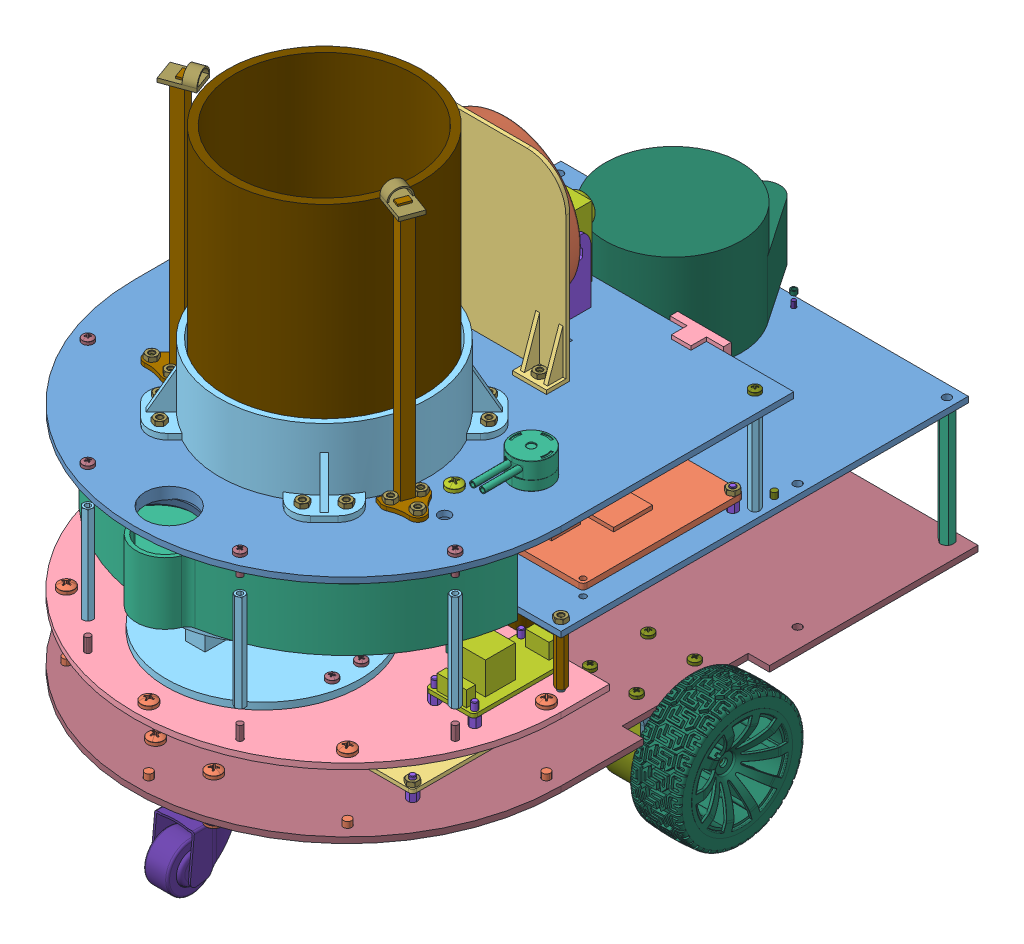
SolidWorks assembly 总装配, configuration 默认. Lengths in mm.
Overall size (259.72 318.06 332.82).
184 component instances, 44 part files, 87 mates.
Components (placement in the parent):
- 中层结构装配-1: 中层结构装配 [默认] at (0 31.5 0) size (220 94.26 332.82)
  - 支撑件_上部-1: 支撑件_上部 [默认] at (0 31 0) size (210 3 210)
  - stm32开发板51_2×82_8-1: stm32开发板51_2×82_8 [默认] at (72.18 39 -65) size (51.24 5 82.8)
  - 6490开发板100×130×39.25-1: 6490开发板100×130×39.25 [默认] at (-40 39 -65) x (0 0 -1) z (1 0 0) size (107 40.25 130)
  - 支撑件_最底部-2: 支撑件_最底部 [默认] at origin size (220 3 135)
  - 压力传感器100-1: 压力传感器100 [默认] at (0 6 43.5) x (0 0 -1) z (1 0 0) size (100 38.5 100)
  - 蓄水容器-1: 蓄水容器 [默认] at (0 44.5 60) size (194.98 32 99)
  - 继电器50x25x18.5-1: 继电器50x25x18.5 [默认] at (83.25 8 5.75) x (0 0 1) z (-1 0 0) size (50 18.5 25)
  - 单通六角螺柱M3-L5]-1: 单通六角螺柱M3-L5] [默认] at (-100 45 -110) x (0 -1 0) z (0 0 1) size (11 5.32 5.32)
  - 单通六角螺柱M3-L5]-2: 单通六角螺柱M3-L5] [默认] at (-100 45 -20) x (0 -1 0) z (0.188455 0 0.982082) size (11 5.32 5.32)
  - 单通六角螺柱M3-L5]-3: 单通六角螺柱M3-L5] [默认] at (20 45 -110) x (0 -1 0) z (0.395734 0 0.918365) size (11 5.32 5.32)
  - 单通六角螺柱M3-L5]-4: 单通六角螺柱M3-L5] [默认] at (20 45 -20) x (0 -1 0) z (0.6 0 0.8) size (11 5.32 5.32)
  - 双通六角螺柱M3-L25]-1: 双通六角螺柱M3-L25] [默认] at (-100 17 -10) x (0 1 0) z (-0.516013 0 0.856581) size (25.01 5.44 5.43)
  - 双通六角螺柱M3-L25]-2: 双通六角螺柱M3-L25] [默认] at (100 17 -10) x (0 1 0) z (-0.345341 0 0.938477) size (25.01 5.44 5.43)
  - 双通六角螺柱M3-L25]-4: 双通六角螺柱M3-L25] [默认] at (0 17 -10) x (0 1 0) z (-0.345341 0 0.938477) size (25.01 5.44 5.43)
  - 蓄水容器盖子-1: 蓄水容器盖子 [默认] at (0 77.4896 10) x (1 0 0) z (0 0 -1) size (194.98 5 80)
  - GB╱T 818-2016[十字槽盘头螺钉M3×4]-1: GB╱T 818-2016[十字槽盘头螺钉M3×4] [默认] at (-100 28.6 -110) x (0 1 0) z (0 0 1) size (6.35 5.6 5.6)
  - 六角螺母 SLMNA[SLMNA-M3]-1: 六角螺母 SLMNA[SLMNA-M3] [默认] at (-100 42 -110) x (1 0 0) z (0 1 0) size (5.5 6.35 2.41)
  - GB╱T 818-2016[十字槽盘头螺钉M3×4]-2: GB╱T 818-2016[十字槽盘头螺钉M3×4] [默认] at (-100 28.6 -20) x (0 1 0) z (0.188455 0 0.982082) size (6.35 5.6 5.6)
  - 六角螺母 SLMNA[SLMNA-M3]-2: 六角螺母 SLMNA[SLMNA-M3] [默认] at (-100 42 -20) x (0.982082 0 -0.188455) z (0 1 0) size (5.5 6.35 2.41)
  - GB╱T 818-2016[十字槽盘头螺钉M3×4]-4: GB╱T 818-2016[十字槽盘头螺钉M3×4] [默认] at (20 28.6 -110) x (0 1 0) z (0.395734 0 0.918365) size (6.35 5.6 5.6)
  - 六角螺母 SLMNA[SLMNA-M3]-4: 六角螺母 SLMNA[SLMNA-M3] [默认] at (20 42 -110) x (0.918365 0 -0.395734) z (0 1 0) size (5.5 6.35 2.41)
  - GB╱T 818-2016[十字槽盘头螺钉M3×4]-6: GB╱T 818-2016[十字槽盘头螺钉M3×4] [默认] at (20 28.6 -20) x (0 1 0) z (0.6 0 0.8) size (6.35 5.6 5.6)
  - 六角螺母 SLMNA[SLMNA-M3]-6: 六角螺母 SLMNA[SLMNA-M3] [默认] at (20 42 -20) x (0.8 0 -0.6) z (0 1 0) size (5.5 6.35 2.41)
  - GB╱T 818-2016[十字槽盘头螺钉M3×10]-1: GB╱T 818-2016[十字槽盘头螺钉M3×10] [默认] at (43 11.9 36) x (0 -1 0) z (-0.546944 0 0.837169) size (12.35 5.6 5.6)
  - GB╱T 818-2016[十字槽盘头螺钉M3×10]-2: GB╱T 818-2016[十字槽盘头螺钉M3×10] [默认] at (43 11.9 51) x (0 -1 0) z (-0.379375 0 0.925243) size (12.35 5.6 5.6)
  - GB╱T 818-2016[十字槽盘头螺钉M3×8]-2: GB╱T 818-2016[十字槽盘头螺钉M3×8] [默认] at (100 -2.4 -10) x (0 1 0) z (0.546944 0 -0.837169) size (10.35 5.6 5.6)
  - 六角螺母 SLMNA[SLMNA-M3]-9: 六角螺母 SLMNA[SLMNA-M3] [默认] at (100 34 -10) x (1 0 0) z (0 1 0) size (5.5 6.35 2.41)
  - 六角螺母 SLMNA[SLMNA-M3]-10: 六角螺母 SLMNA[SLMNA-M3] [默认] at (0 34 -10) x (0.982082 0 -0.188455) z (0 1 0) size (5.5 6.35 2.41)
  - GB╱T 818-2016[十字槽盘头螺钉M3×8]-3: GB╱T 818-2016[十字槽盘头螺钉M3×8] [默认] at (0 -2.4 -10) x (0 1 0) z (0.379375 0 -0.925243) size (10.35 5.6 5.6)
  - 六角螺母 SLMNA[SLMNA-M3]-14: 六角螺母 SLMNA[SLMNA-M3] [默认] at (-100 34 -10) x (0.92897 0 -0.370156) z (0 1 0) size (5.5 6.35 2.41)
  - GB╱T 818-2016[十字槽盘头螺钉M3×8]-6: GB╱T 818-2016[十字槽盘头螺钉M3×8] [默认] at (-100 -2.4 -10) x (0 1 0) z (0.198211 0 -0.980159) size (10.35 5.6 5.6)
  - 单通六角螺柱M3-L5]-5: 单通六角螺柱M3-L5] [默认] at (93.5 14 28) x (0 -1 0) z (-0.997819 0 -0.066013) size (11 5.32 5.32)
  - 单通六角螺柱M3-L5]-6: 单通六角螺柱M3-L5] [默认] at (73 14 28) x (0 -1 0) z (-0.99238 0 0.123213) size (11 5.32 5.32)
  - 单通六角螺柱M3-L5]-7: 单通六角螺柱M3-L5] [默认] at (93.5 14 -16.5) x (0 -1 0) z (-0.942486 0 0.334247) size (11 5.32 5.32)
  - 单通六角螺柱M3-L5]-8: 单通六角螺柱M3-L5] [默认] at (73 14 -16.5) x (0 -1 0) z (-0.837863 0 0.545881) size (11 5.32 5.32)
  - 雷达-2: 雷达 [默认] at (0 36.9114 -167.8168) x (0 0 -1) z (1 0 0) size (90 52 70)
  - 单通六角螺柱M3-L5]-10: 单通六角螺柱M3-L5] [默认] at (95 45 -103.6) x (0 -1 0) z (-0.546944 0 0.837169) size (11 5.32 5.32)
  - 六角螺母 SLMNA[SLMNA-M3]-15: 六角螺母 SLMNA[SLMNA-M3] [默认] at (95 44.4 -103.6) x (1 0 0) z (0 -1 0) size (5.5 6.35 2.41)
  - GB╱T 818-2016[十字槽盘头螺钉M3×6]-1: GB╱T 818-2016[十字槽盘头螺钉M3×6] [默认] at (95 28.6 -103.6) x (0 1 0) z (0 0 1) size (8.35 5.6 5.6)
  - GB╱T 818-2016[十字槽盘头螺钉M2×6]-1: GB╱T 818-2016[十字槽盘头螺钉M2×6] [默认] at (20 29.4 -210) x (0 1 0) z (-0.975796 0 -0.218684) size (7.56 4 4)
- 上层支撑结构-1: 上层支撑结构 [默认] at (0 116.5 0) size (220 164.3 234)
  - 花盆100×100×130-1: 花盆100×100×130 [默认] at (0 1 12) size (100 130 100)
  - 支撑件_最顶部-1: 支撑件_最顶部 [默认] x (-1 0 0) z (0 0 1) size (220 6 230)
  - 一体化麦-1: 一体化麦 [默认] at (0 49.5771 -67) x (1 0 0) z (0 1 0) size (88 15 88)
  - 上层竖直安装版-1: 上层竖直安装版 [默认] at (0 48.5 -67) size (95 95 12)
  - 0.96寸led大概-1: 0.96寸led大概 [默认] at (60 -10.65 -120) x (-1 0 0) z (0 0 -1) size (27.6 27.3 12)
  - 0.96寸led大概-3: 0.96寸led大概 [默认] at (-60 -10.65 -120) x (-1 0 0) z (0 0 -1) size (27.6 27.3 12)
  - 花盆支撑-1: 花盆支撑 [默认] at (-36.7696 1 48.7696) x (0.707107 0 -0.707107) z (0.707107 0 0.707107) size (134 35 134)
  - 蠕动泵-1: 蠕动泵 [默认] at (20.9584 -7.5 -18.6981) x (0 0 1) z (0 1 0) size (38.31 20 40.3)
  - 相机-1: 相机 [默认] at (0 28.3524 -102.4535) x (-1 0 0) z (0 0 -1) size (36 36 25.5)
  - 相机支架-1: 相机支架 [默认] at (0 1 -100) size (40.08 35.04 25)
  - 花盆引导架-1: 花盆引导架 [默认] at (62 1 30) x (0.939693 0 0.34202) z (-0.34202 0 0.939693) size (18.5 133 20.12)
  - 花盆引导架-2: 花盆引导架 [默认] at (-62 1 30) x (-0.939693 0 0.34202) z (-0.34202 0 -0.939693) size (18.5 133 20.12)
  - GB╱T 818-2016[十字槽盘头螺钉M3×6]-1: GB╱T 818-2016[十字槽盘头螺钉M3×6] [默认] at (68.5778 -4.4 32.3941) x (0 1 0) z (0 0 1) size (8.35 5.6 5.6)
  - GB╱T 818-2016[十字槽盘头螺钉M3×6]-2: GB╱T 818-2016[十字槽盘头螺钉M3×6] [默认] at (56.6377 -4.4 34.4995) x (0 1 0) z (0.188455 0 0.982082) size (8.35 5.6 5.6)
  - GB╱T 818-2016[十字槽盘头螺钉M3×6]-5: GB╱T 818-2016[十字槽盘头螺钉M3×6] [默认] at (60.7845 -4.4 23.1063) x (0 1 0) z (0.370156 0 0.92897) size (8.35 5.6 5.6)
  - GB╱T 818-2016[十字槽盘头螺钉M3×6]-7: GB╱T 818-2016[十字槽盘头螺钉M3×6] [默认] at (-56.6377 -4.4 34.4995) x (0 1 0) z (0.561714 0 0.827332) size (8.35 5.6 5.6)
  - GB╱T 818-2016[十字槽盘头螺钉M3×6]-10: GB╱T 818-2016[十字槽盘头螺钉M3×6] [默认] at (-68.5778 -4.4 32.3941) x (0 1 0) z (0.707564 0 0.70665) size (8.35 5.6 5.6)
  - GB╱T 818-2016[十字槽盘头螺钉M3×6]-12: GB╱T 818-2016[十字槽盘头螺钉M3×6] [默认] at (-60.7845 -4.4 23.1063) x (0 1 0) z (0.843262 0 0.537503) size (8.35 5.6 5.6)
  - GB╱T 818-2016[十字槽盘头螺钉M3×6]-14: GB╱T 818-2016[十字槽盘头螺钉M3×6] [默认] at (-36.7696 -4.4 60.0833) x (0 1 0) z (0.94577 0 0.324837) size (8.35 5.6 5.6)
  - GB╱T 818-2016[十字槽盘头螺钉M3×6]-16: GB╱T 818-2016[十字槽盘头螺钉M3×6] [默认] at (-48.0833 -4.4 48.7696) x (0 1 0) z (0.995978 0 0.089595) size (8.35 5.6 5.6)
  - GB╱T 818-2016[十字槽盘头螺钉M3×6]-18: GB╱T 818-2016[十字槽盘头螺钉M3×6] [默认] at (-48.0833 -4.4 -24.7696) x (0 1 0) z (0.990656 0 -0.136386) size (8.35 5.6 5.6)
  - GB╱T 818-2016[十字槽盘头螺钉M3×6]-20: GB╱T 818-2016[十字槽盘头螺钉M3×6] [默认] at (-36.7696 -4.4 -36.0833) x (0 1 0) z (0.100159 0 0.994971) size (8.35 5.6 5.6)
  - GB╱T 818-2016[十字槽盘头螺钉M3×6]-23: GB╱T 818-2016[十字槽盘头螺钉M3×6] [默认] at (36.7696 -4.4 -36.0833) x (0 1 0) z (0.888841 0 -0.458216) size (8.35 5.6 5.6)
  - GB╱T 818-2016[十字槽盘头螺钉M3×6]-25: GB╱T 818-2016[十字槽盘头螺钉M3×6] [默认] at (48.0833 -4.4 -24.7696) x (0 1 0) z (0.844013 0 -0.536322) size (8.35 5.6 5.6)
  - GB╱T 818-2016[十字槽盘头螺钉M3×6]-27: GB╱T 818-2016[十字槽盘头螺钉M3×6] [默认] at (36.7696 -4.4 60.0833) x (0 1 0) z (0.827332 0 -0.561714) size (8.35 5.6 5.6)
  - GB╱T 818-2016[十字槽盘头螺钉M3×6]-29: GB╱T 818-2016[十字槽盘头螺钉M3×6] [默认] at (48.0833 -4.4 48.7696) x (0 1 0) z (0.844013 0 -0.536322) size (8.35 5.6 5.6)
  - 六角螺母 SLMNA[SLMNA-M3]-1: 六角螺母 SLMNA[SLMNA-M3] [默认] at (-48.0833 6.4 48.7696) x (1 0 0) z (0 -1 0) size (5.5 6.35 2.41)
  - 六角螺母 SLMNA[SLMNA-M3]-2: 六角螺母 SLMNA[SLMNA-M3] [默认] at (-36.7696 6.4 60.0833) x (0.982082 0 -0.188455) z (0 -1 0) size (5.5 6.35 2.41)
  - 六角螺母 SLMNA[SLMNA-M3]-4: 六角螺母 SLMNA[SLMNA-M3] [默认] at (-68.5778 5.4 32.3941) x (0.918365 0 -0.395734) z (0 -1 0) size (5.5 6.35 2.41)
  - 六角螺母 SLMNA[SLMNA-M3]-6: 六角螺母 SLMNA[SLMNA-M3] [默认] at (-60.7845 5.4 23.1063) x (0.8 0 -0.6) z (0 -1 0) size (5.5 6.35 2.41)
  - 六角螺母 SLMNA[SLMNA-M3]-8: 六角螺母 SLMNA[SLMNA-M3] [默认] at (-56.6377 5.4 34.4995) x (0.63358 0 -0.773678) z (0 -1 0) size (5.5 6.35 2.41)
  - 六角螺母 SLMNA[SLMNA-M3]-10: 六角螺母 SLMNA[SLMNA-M3] [默认] at (56.6377 5.4 34.4995) x (0.443629 0 -0.896211) z (0 -1 0) size (5.5 6.35 2.41)
  - 六角螺母 SLMNA[SLMNA-M3]-12: 六角螺母 SLMNA[SLMNA-M3] [默认] at (68.5778 5.4 32.3941) x (0.263225 0 -0.964735) z (0 -1 0) size (5.5 6.35 2.41)
  - 六角螺母 SLMNA[SLMNA-M3]-14: 六角螺母 SLMNA[SLMNA-M3] [默认] at (60.7845 5.4 23.1063) x (0.120178 0 -0.992752) z (0 -1 0) size (5.5 6.35 2.41)
  - 六角螺母 SLMNA[SLMNA-M3]-16: 六角螺母 SLMNA[SLMNA-M3] [默认] at (48.0833 6.4 48.7696) x (0.030377 0 -0.999538) z (0 -1 0) size (5.5 6.35 2.41)
  - 六角螺母 SLMNA[SLMNA-M3]-18: 六角螺母 SLMNA[SLMNA-M3] [默认] at (36.7696 6.4 60.0833) x (0 0 -1) z (0 -1 0) size (5.5 6.35 2.41)
  - 六角螺母 SLMNA[SLMNA-M3]-20: 六角螺母 SLMNA[SLMNA-M3] [默认] at (48.0833 6.4 -24.7696) x (0.030377 0 -0.999538) z (0 -1 0) size (5.5 6.35 2.41)
  - 六角螺母 SLMNA[SLMNA-M3]-22: 六角螺母 SLMNA[SLMNA-M3] [默认] at (36.7696 6.4 -36.0833) x (0.120178 0 -0.992752) z (0 -1 0) size (5.5 6.35 2.41)
  - 六角螺母 SLMNA[SLMNA-M3]-24: 六角螺母 SLMNA[SLMNA-M3] [默认] at (-48.0833 6.4 -24.7696) x (0.263225 0 -0.964735) z (0 -1 0) size (5.5 6.35 2.41)
  - 六角螺母 SLMNA[SLMNA-M3]-26: 六角螺母 SLMNA[SLMNA-M3] [默认] at (-36.7696 6.4 -36.0833) x (0.95137 0 -0.308051) z (0 -1 0) size (5.5 6.35 2.41)
  - 六角螺母 SLMNA[SLMNA-M3]-30: 六角螺母 SLMNA[SLMNA-M3] [默认] at (-39 5.4 -60) x (0.95137 0 -0.308051) z (0 -1 0) size (5.5 6.35 2.41)
  - 六角螺母 SLMNA[SLMNA-M3]-31: 六角螺母 SLMNA[SLMNA-M3] [默认] at (39 5.4 -60) x (0.876269 0 -0.481821) z (0 -1 0) size (5.5 6.35 2.41)
  - GB╱T 818-2016[十字槽盘头螺钉M3×6]-32: GB╱T 818-2016[十字槽盘头螺钉M3×6] [默认] at (-39 -4.4 -60) x (0 1 0) z (0.84405 0 -0.536264) size (8.35 5.6 5.6)
  - GB╱T 818-2016[十字槽盘头螺钉M3×6]-33: GB╱T 818-2016[十字槽盘头螺钉M3×6] [默认] at (39 -4.4 -60) x (0 1 0) z (0.727865 0 -0.685721) size (8.35 5.6 5.6)
  - GB╱T 818-2016[十字槽盘头螺钉M6×8]-1: GB╱T 818-2016[十字槽盘头螺钉M6×8] [默认] at (0 7.6 -100) x (0 -1 0) z (-0.546944 0 0.837169) size (12.48 12 12)
  - 六角螺母 SLMNA[SLMNA-M6]-1: 六角螺母 SLMNA[SLMNA-M6] [默认] at (0 -2 -100) x (1 0 0) z (0 -1 0) size (11.55 11.55 5.01)
  - 引导平台-1: 引导平台 [默认] at (56.5968 131 28.0334) x (-0.939693 0 -0.34202) z (0.34202 0 -0.939693) size (16 7.5 11)
  - 引导平台-2: 引导平台 [默认] at (-56.5968 131 28.0334) x (0.939693 0 -0.34202) z (0.34202 0 0.939693) size (16 7.5 11)
- 底部驱动层-1: 底部驱动层 [默认] at origin size (259.72 106.58 325)
  - 底架-2: 底架 [默认] at origin size (220 3 325)
  - MG513电机支架-2: MG513电机支架 [默认] at (76.5 -1.5 -75) x (0 0 -1) z (0 -1 0) size (40 41 47)
  - 65mm车轮-1: 65mm车轮 [默认] at (115.38 -21.2 -75) x (0 -0.304944 0.95237) z (0 -0.95237 -0.304944) size (66.59 27.57 66.59)
  - MG513P3012V电机-1: MG513P3012V电机 [默认] at (96 -28.5 -75) x (0 -1 0) z (0 0 1) size (36.6 72.9 36.6)
  - 65mm车轮-2: 65mm车轮 [默认] at (-115.38 -21.2 -75) x (0 0.304944 -0.95237) z (0 -0.95237 -0.304944) size (66.59 27.57 66.59)
  - MG513P3012V电机-2: MG513P3012V电机 [默认] at (-96 -28.5 -75) x (0 -1 0) z (0 0 -1) size (36.6 72.9 36.6)
  - MG513电机支架-3: MG513电机支架 [默认] at (-76.5 -1.5 -75) x (0 0 1) z (0 -1 0) size (40 41 47)
  - 1寸万向轮(30X24)-1: 1寸万向轮(30X24) [默认] at (0 -18.5 72) x (-1 0 0) z (0 1 0) size (39 43.5 38.5)
  - E351S电池-1: E351S电池 [默认] at (0 1.5 -79.3271) x (0 0 -1) z (0 1 0) size (72.6 85.6 42.03)
  - 单通六角螺柱M3-L5]-1: 单通六角螺柱M3-L5] [默认] at (-11 -4.5 -14) x (0 1 0) z (-0.004177 0 -0.999991) size (11 5.32 5.32)
  - 双通六角螺柱M4-L16]-1: 双通六角螺柱M4-L16] [默认] at (15 -9.5 84) x (0 -1 0) z (0.861401 0 -0.507926) size (16.01 6.94 6.93)
  - 双通六角螺柱M4-L16]-2: 双通六角螺柱M4-L16] [默认] at (-15 -9.5 84) x (0 -1 0) z (0.988419 0 0.15175) size (16.01 6.94 6.93)
  - 双通六角螺柱M4-L16]-3: 双通六角螺柱M4-L16] [默认] at (-15 -9.5 60) x (0 -1 0) z (0.997892 0 -0.064894) size (16.01 6.94 6.93)
  - 双通六角螺柱M4-L16]-4: 双通六角螺柱M4-L16] [默认] at (15 -9.5 60) x (0 -1 0) z (0.95487 0 -0.297023) size (16.01 6.94 6.93)
  - GB╱T 818-2000[十字槽盘头螺钉M4×6]-1: GB╱T 818-2000[十字槽盘头螺钉M4×6] [默认] at (-15 4.6 84) x (0 -1 0) z (-0.891014 0 0.453975) size (9.03 8 8)
  - GB╱T 818-2000[十字槽盘头螺钉M4×6]-2: GB╱T 818-2000[十字槽盘头螺钉M4×6] [默认] at (-15 4.6 60) x (0 -1 0) z (-0.52314 0 0.852247) size (9.03 8 8)
  - GB╱T 818-2000[十字槽盘头螺钉M4×6]-3: GB╱T 818-2000[十字槽盘头螺钉M4×6] [默认] at (15 4.6 60) x (0 -1 0) z (-0.327118 0 0.944983) size (9.03 8 8)
  - GB╱T 818-2000[十字槽盘头螺钉M4×6]-4: GB╱T 818-2000[十字槽盘头螺钉M4×6] [默认] at (15 4.6 84) x (0 -1 0) z (-0.096468 0 0.995336) size (9.03 8 8)
  - GB╱T 818-2000[十字槽盘头螺钉M4×6]-7: GB╱T 818-2000[十字槽盘头螺钉M4×6] [默认] at (-15 -21.6 84) x (0 1 0) z (0.029897 0 0.999553) size (9.03 8 8)
  - GB╱T 818-2000[十字槽盘头螺钉M4×6]-8: GB╱T 818-2000[十字槽盘头螺钉M4×6] [默认] at (-15 -21.6 60) x (0 1 0) z (0.217732 0 0.976009) size (9.03 8 8)
  - GB╱T 818-2000[十字槽盘头螺钉M4×6]-9: GB╱T 818-2000[十字槽盘头螺钉M4×6] [默认] at (15 -21.6 60) x (0 1 0) z (0.423014 0 0.906123) size (9.03 8 8)
  - GB╱T 818-2000[十字槽盘头螺钉M4×6]-10: GB╱T 818-2000[十字槽盘头螺钉M4×6] [默认] at (15 -21.6 84) x (0 1 0) z (0.62365 0 0.781704) size (9.03 8 8)
  - 单通六角螺柱M3-L5]-2: 单通六角螺柱M3-L5] [默认] at (-11 -4.5 30) x (0 1 0) z (0.144289 0 -0.989536) size (11 5.32 5.32)
  - 单通六角螺柱M3-L5]-3: 单通六角螺柱M3-L5] [默认] at (-55 -4.5 30) x (0 1 0) z (-0.351214 0 -0.936295) size (11 5.32 5.32)
  - 单通六角螺柱M3-L5]-4: 单通六角螺柱M3-L5] [默认] at (-55 -4.5 -14) x (0 1 0) z (-0.646465 0 -0.762944) size (11 5.32 5.32)
  - 六角螺母 SLMNA[SLMNA-M3]-1: 六角螺母 SLMNA[SLMNA-M3] [默认] at (-55 -1.5 -14) x (1 0 0) z (0 -1 0) size (5.5 6.35 2.41)
  - GB╱T 818-2016[十字槽盘头螺钉M3×4]-1: GB╱T 818-2016[十字槽盘头螺钉M3×4] [默认] at (-55 10.9039 -14) x (0 -1 0) z (0 0 1) size (6.35 5.6 5.6)
  - GB╱T 818-2016[十字槽盘头螺钉M3×4]-3: GB╱T 818-2016[十字槽盘头螺钉M3×4] [默认] at (-55 10.4 30) x (0 -1 0) z (0.188455 0 0.982082) size (6.35 5.6 5.6)
  - 六角螺母 SLMNA[SLMNA-M3]-3: 六角螺母 SLMNA[SLMNA-M3] [默认] at (-55 -1.5 30) x (0.982082 0 -0.188455) z (0 -1 0) size (5.5 6.35 2.41)
  - GB╱T 818-2016[十字槽盘头螺钉M3×4]-5: GB╱T 818-2016[十字槽盘头螺钉M3×4] [默认] at (-11 10.4 30) x (0 -1 0) z (0.278271 0 0.960503) size (6.35 5.6 5.6)
  - 六角螺母 SLMNA[SLMNA-M3]-5: 六角螺母 SLMNA[SLMNA-M3] [默认] at (-11 -1.5 30) x (0.918365 0 -0.395734) z (0 -1 0) size (5.5 6.35 2.41)
  - GB╱T 818-2016[十字槽盘头螺钉M3×4]-7: GB╱T 818-2016[十字槽盘头螺钉M3×4] [默认] at (-11 10.4 -14) x (0 -1 0) z (0.715828 0 0.698276) size (6.35 5.6 5.6)
  - 六角螺母 SLMNA[SLMNA-M3]-7: 六角螺母 SLMNA[SLMNA-M3] [默认] at (-11 -1.5 -14) x (0.8 0 -0.6) z (0 -1 0) size (5.5 6.35 2.41)
  - GB╱T 818-2016[十字槽盘头螺钉M3×6]-1: GB╱T 818-2016[十字槽盘头螺钉M3×6] [默认] at (-65 3.9 -90) x (0 -1 0) z (-0.884583 0 -0.466383) size (8.35 5.6 5.6)
  - 六角螺母 SLMNA[SLMNA-M3]-9: 六角螺母 SLMNA[SLMNA-M3] [默认] at (-65 -3.5 -90) x (1 0 0) z (0 -1 0) size (5.5 6.35 2.41)
  - 六角螺母 SLMNA[SLMNA-M3]-10: 六角螺母 SLMNA[SLMNA-M3] [默认] at (-65 -3.5 -60) x (0.982082 0 -0.188455) z (0 -1 0) size (5.5 6.35 2.41)
  - GB╱T 818-2016[十字槽盘头螺钉M3×6]-2: GB╱T 818-2016[十字槽盘头螺钉M3×6] [默认] at (-65 3.9 -60) x (0 -1 0) z (-0.997848 0 0.065565) size (8.35 5.6 5.6)
  - 六角螺母 SLMNA[SLMNA-M3]-12: 六角螺母 SLMNA[SLMNA-M3] [默认] at (-89 -3.5 -60) x (0.918365 0 -0.395734) z (0 -1 0) size (5.5 6.35 2.41)
  - GB╱T 818-2016[十字槽盘头螺钉M3×6]-4: GB╱T 818-2016[十字槽盘头螺钉M3×6] [默认] at (-89 3.9 -60) x (0 -1 0) z (0.679872 0 0.733331) size (8.35 5.6 5.6)
  - 六角螺母 SLMNA[SLMNA-M3]-14: 六角螺母 SLMNA[SLMNA-M3] [默认] at (-89 -3.5 -90) x (0.8 0 -0.6) z (0 -1 0) size (5.5 6.35 2.41)
  - GB╱T 818-2016[十字槽盘头螺钉M3×6]-6: GB╱T 818-2016[十字槽盘头螺钉M3×6] [默认] at (-89 3.9 -90) x (0 -1 0) z (-0.990123 0 0.140204) size (8.35 5.6 5.6)
  - 六角螺母 SLMNA[SLMNA-M3]-16: 六角螺母 SLMNA[SLMNA-M3] [默认] at (65 -3.5 -90) x (0.63358 0 -0.773678) z (0 -1 0) size (5.5 6.35 2.41)
  - GB╱T 818-2016[十字槽盘头螺钉M3×6]-8: GB╱T 818-2016[十字槽盘头螺钉M3×6] [默认] at (65 3.9 -90) x (0 -1 0) z (-0.999945 0 -0.010447) size (8.35 5.6 5.6)
  - 六角螺母 SLMNA[SLMNA-M3]-18: 六角螺母 SLMNA[SLMNA-M3] [默认] at (89 -2 -90) x (0.443629 0 -0.896211) z (0 -1 0) size (5.5 6.35 2.41)
  - GB╱T 818-2016[十字槽盘头螺钉M3×6]-10: GB╱T 818-2016[十字槽盘头螺钉M3×6] [默认] at (89 3.9 -90) x (0 -1 0) z (-0.507639 0 -0.86157) size (8.35 5.6 5.6)
  - 六角螺母 SLMNA[SLMNA-M3]-20: 六角螺母 SLMNA[SLMNA-M3] [默认] at (65 -3.5 -60) x (0.263225 0 -0.964735) z (0 -1 0) size (5.5 6.35 2.41)
  - GB╱T 818-2016[十字槽盘头螺钉M3×6]-12: GB╱T 818-2016[十字槽盘头螺钉M3×6] [默认] at (65 3.9 -60) x (0 -1 0) z (-0.663677 0 -0.748019) size (8.35 5.6 5.6)
  - 六角螺母 SLMNA[SLMNA-M3]-22: 六角螺母 SLMNA[SLMNA-M3] [默认] at (89 -3.5 -60) x (0.120178 0 -0.992752) z (0 -1 0) size (5.5 6.35 2.41)
  - GB╱T 818-2016[十字槽盘头螺钉M3×6]-14: GB╱T 818-2016[十字槽盘头螺钉M3×6] [默认] at (89 3.9 -60) x (0 -1 0) z (-0.765371 0 -0.643589) size (8.35 5.6 5.6)
  - 稳压电源模块-1: 稳压电源模块 [默认] at (58.75 6.5 13.25) x (0 0 -1) z (1 0 0) size (68 12 44)
  - 单通六角螺柱M3-L5]-5: 单通六角螺柱M3-L5] [默认] at (77.5 12.5 44) x (0 -1 0) z (-0.177276 0 0.984161) size (11 5.32 5.32)
  - 六角螺母 SLMNA[SLMNA-M3]-23: 六角螺母 SLMNA[SLMNA-M3] [默认] at (77.5 10.9 44) x (1 0 0) z (0 -1 0) size (5.5 6.35 2.41)
  - GB╱T 818-2016[十字槽盘头螺钉M3×4]-8: GB╱T 818-2016[十字槽盘头螺钉M3×4] [默认] at (77.5 -3.9 44) x (0 1 0) z (-0.488531 0 0.872547) size (6.35 5.6 5.6)
  - tb6612 50×50-1: tb6612 50×50 [默认] at (-33 6.5 8) size (50 1.5 50)
- 双通六角螺柱M3-L50]-1: 双通六角螺柱M3-L50] [默认] at (-94.6977 74.5 39.2251) x (0 1 0) z (0.093168 0 0.99565) size (50.01 5.44 5.43)
- 双通六角螺柱M3-L50]-2: 双通六角螺柱M3-L50] [默认] at (-39.2251 74.5 94.6977) x (0 1 0) z (0.279133 0 0.960252) size (50.01 5.44 5.43)
- 双通六角螺柱M3-L50]-3: 双通六角螺柱M3-L50] [默认] at (39.2251 74.5 94.6977) x (0 1 0) z (0.479575 0 0.877501) size (50.01 5.44 5.43)
- 双通六角螺柱M3-L50]-4: 双通六角螺柱M3-L50] [默认] at (94.6977 74.5 39.2251) x (0 1 0) z (0.9746 0 -0.223951) size (50.01 5.44 5.43)
- 双通六角螺柱M4-L60]-1: 双通六角螺柱M4-L60] [默认] at (-65 74.5 10) x (0 -1 0) z (-0.823927 0 0.566696) size (60.01 6.94 6.93)
- 双通六角螺柱M4-L60]-4: 双通六角螺柱M4-L60] [默认] at (65 74.5 10) x (0 -1 0) z (-0.703105 0 0.711086) size (60.01 6.94 6.93)
- 双通六角螺柱M3-L50]-11: 双通六角螺柱M3-L50] [默认] at (-100 90.5 -110) x (0 -1 0) z (0.626129 0 0.779719) size (50.01 5.44 5.43)
- 双通六角螺柱M3-L50]-13: 双通六角螺柱M3-L50] [默认] at (100 90.5 -110) x (0 -1 0) z (0.761852 0 0.647751) size (50.01 5.44 5.43)
- GB╱T 818-2000[十字槽盘头螺钉M4×6]-1: GB╱T 818-2000[十字槽盘头螺钉M4×6] [默认] at (-102.5 -4.6 0) x (0 1 0) z (-0.546493 0 -0.837464) size (9.03 8 8)
- GB╱T 818-2000[十字槽盘头螺钉M4×6]-2: GB╱T 818-2000[十字槽盘头螺钉M4×6] [默认] at (-102.5 37.6 0) x (0 -1 0) z (-0.612652 0 -0.790353) size (9.03 8 8)
- GB╱T 818-2000[十字槽盘头螺钉M4×6]-3: GB╱T 818-2000[十字槽盘头螺钉M4×6] [默认] at (-72.4784 37.6 72.4784) x (0 -1 0) z (-0.75062 0 -0.660734) size (9.03 8 8)
- GB╱T 818-2000[十字槽盘头螺钉M4×6]-4: GB╱T 818-2000[十字槽盘头螺钉M4×6] [默认] at (-72.4784 -4.6 72.4784) x (0 1 0) z (-0.694525 0 -0.719469) size (9.03 8 8)
- GB╱T 818-2000[十字槽盘头螺钉M4×6]-5: GB╱T 818-2000[十字槽盘头螺钉M4×6] [默认] at (0 37.6 102.5) x (0 -1 0) z (-0.875408 0 -0.483385) size (9.03 8 8)
- GB╱T 818-2000[十字槽盘头螺钉M4×6]-6: GB╱T 818-2000[十字槽盘头螺钉M4×6] [默认] at (0 -4.6 102.5) x (0 1 0) z (-0.833293 0 -0.552832) size (9.03 8 8)
- GB╱T 818-2000[十字槽盘头螺钉M4×6]-7: GB╱T 818-2000[十字槽盘头螺钉M4×6] [默认] at (72.4784 37.6 72.4784) x (0 -1 0) z (-0.964333 0 -0.264691) size (9.03 8 8)
- GB╱T 818-2000[十字槽盘头螺钉M4×6]-8: GB╱T 818-2000[十字槽盘头螺钉M4×6] [默认] at (72.4784 -4.6 72.4784) x (0 1 0) z (-0.939673 0 -0.342075) size (9.03 8 8)
- GB╱T 818-2000[十字槽盘头螺钉M4×6]-9: GB╱T 818-2000[十字槽盘头螺钉M4×6] [默认] at (102.5 37.6 0) x (0 -1 0) z (-0.999642 0 -0.026756) size (9.03 8 8)
- GB╱T 818-2000[十字槽盘头螺钉M4×6]-13: GB╱T 818-2000[十字槽盘头螺钉M4×6] [默认] at (102.5 -4.6 0) x (0 1 0) z (-0.987301 0 -0.15886) size (9.03 8 8)
- GB╱T 818-2016[十字槽盘头螺钉M3×6]-9: GB╱T 818-2016[十字槽盘头螺钉M3×6] [默认] at (100 60.1 -120) x (0 1 0) z (0.177827 0 0.984062) size (8.35 5.6 5.6)
- GB╱T 818-2016[十字槽盘头螺钉M3×6]-10: GB╱T 818-2016[十字槽盘头螺钉M3×6] [默认] at (100 119.9 -110) x (0 -1 0) z (1 0 0) size (8.35 5.6 5.6)
- GB╱T 818-2016[十字槽盘头螺钉M3×6]-13: GB╱T 818-2016[十字槽盘头螺钉M3×6] [默认] at (-100 60.1 -120) x (0 1 0) z (-0.038492 0 0.999259) size (8.35 5.6 5.6)
- GB╱T 818-2016[十字槽盘头螺钉M3×6]-14: GB╱T 818-2016[十字槽盘头螺钉M3×6] [默认] at (-100 119.9 -110) x (0 -1 0) z (1 0 0) size (8.35 5.6 5.6)
- GB╱T 818-2016[十字槽盘头螺钉M4×8]-1: GB╱T 818-2016[十字槽盘头螺钉M4×8] [默认] at (-65 28.4 10) x (0 1 0) z (0.297126 0 0.954838) size (11.03 8 8)
- GB╱T 818-2016[十字槽盘头螺钉M4×8]-2: GB╱T 818-2016[十字槽盘头螺钉M4×8] [默认] at (-65 120.6 10) x (0 -1 0) z (0.954838 0 0.297126) size (11.03 8 8)
- GB╱T 818-2016[十字槽盘头螺钉M4×8]-8: GB╱T 818-2016[十字槽盘头螺钉M4×8] [默认] at (65 28.4 10) x (0 1 0) z (0.810604 0 0.585595) size (11.03 8 8)
- GB╱T 818-2016[十字槽盘头螺钉M4×8]-9: GB╱T 818-2016[十字槽盘头螺钉M4×8] [默认] at (65 120.6 10) x (0 -1 0) z (0.942146 0 -0.335202) size (11.03 8 8)
- GB╱T 818-2016[十字槽盘头螺钉M3×10]-1: GB╱T 818-2016[十字槽盘头螺钉M3×10] [默认] at (-94.6977 29.1 39.2251) x (0 1 0) z (0 0 1) size (12.35 5.6 5.6)
- GB╱T 818-2016[十字槽盘头螺钉M3×10]-2: GB╱T 818-2016[十字槽盘头螺钉M3×10] [默认] at (-94.6977 119.9 39.2251) x (0 -1 0) z (1 0 0) size (12.35 5.6 5.6)
- GB╱T 818-2016[十字槽盘头螺钉M3×10]-4: GB╱T 818-2016[十字槽盘头螺钉M3×10] [默认] at (-39.2251 29.1 94.6977) x (0 1 0) z (0.395734 0 0.918365) size (12.35 5.6 5.6)
- GB╱T 818-2016[十字槽盘头螺钉M3×10]-5: GB╱T 818-2016[十字槽盘头螺钉M3×10] [默认] at (-39.2251 119.9 94.6977) x (0 -1 0) z (0.918365 0 -0.395734) size (12.35 5.6 5.6)
- GB╱T 818-2016[十字槽盘头螺钉M3×10]-8: GB╱T 818-2016[十字槽盘头螺钉M3×10] [默认] at (39.2251 29.1 94.6977) x (0 1 0) z (0.6 0 0.8) size (12.35 5.6 5.6)
- GB╱T 818-2016[十字槽盘头螺钉M3×10]-9: GB╱T 818-2016[十字槽盘头螺钉M3×10] [默认] at (39.2251 119.9 94.6977) x (0 -1 0) z (0.8 0 -0.6) size (12.35 5.6 5.6)
- GB╱T 818-2016[十字槽盘头螺钉M3×10]-12: GB╱T 818-2016[十字槽盘头螺钉M3×10] [默认] at (94.6977 29.1 39.2251) x (0 1 0) z (0.773678 0 0.63358) size (12.35 5.6 5.6)
- GB╱T 818-2016[十字槽盘头螺钉M3×10]-13: GB╱T 818-2016[十字槽盘头螺钉M3×10] [默认] at (94.6977 119.9 39.2251) x (0 -1 0) z (0.63358 0 -0.773678) size (12.35 5.6 5.6)
- 双通六角螺柱M4-L30]-1: 双通六角螺柱M4-L30] [默认] at (-102.5 16.5 0) x (0 -1 0) z (0 0 1) size (30.01 6.94 6.93)
- 双通六角螺柱M4-L60]-5: 双通六角螺柱M4-L60] [默认] at (-100 31.5 -132) x (0 1 0) z (0 0 1) size (60.01 6.94 6.93)
- GB╱T 818-2000[十字槽盘头螺钉M4×6]-14: GB╱T 818-2000[十字槽盘头螺钉M4×6] [默认] at (-100 68.6 -132) x (0 -1 0) z (0 0 1) size (9.03 8 8)
- 双通六角螺柱M4-L60]-6: 双通六角螺柱M4-L60] [默认] at (-100 31.5 -209) x (0 1 0) z (0.188455 0 0.982082) size (60.01 6.94 6.93)
- 双通六角螺柱M4-L60]-7: 双通六角螺柱M4-L60] [默认] at (100 31.5 -209) x (0 1 0) z (0.395734 0 0.918365) size (60.01 6.94 6.93)
Mates (geometry in assembly coordinates):
- 重合1: coincident aligned: plane of 底部驱动层-1 through (0 0 0) normal (0 0 1)
- 重合2: coincident aligned: plane of 底部驱动层-1 through (0 0 0) normal (0 1 0)
- 重合3: coincident aligned: plane of 底部驱动层-1 through (0 0 0) normal (1 0 0)
- 距离1: distance = 30 mm anti-aligned: plane of 中层结构装配-1/支撑件_最底部-2 through (0 31.5 0) normal (0 -1 0); plane of 底部驱动层-1/底架-2 through (0 1.5 0) normal (0 1 0)
- 重合7: coincident aligned: plane of 中层结构装配-1 through (0 31.5 0) normal (1 0 0)
- 重合8: coincident aligned: plane of 上层支撑结构-1 through (0 116.5 0) normal (1 0 0)
- 同心1: concentric aligned: circle of 中层结构装配-1/支撑件_最底部-2; circle of 底部驱动层-1/底架-2
- 同心3: concentric anti-aligned: circle of 中层结构装配-1/支撑件_最底部-2; circle of 上层支撑结构-1/支撑件_最顶部-1
- 同心10: concentric anti-aligned: circle of 中层结构装配-1/支撑件_最底部-2; circle of 双通六角螺柱M3-L50]-1
- 距离2: distance = 15 mm anti-aligned: plane of 双通六角螺柱M3-L50]-1 through (-94.6977 49.5 39.2251) normal (0 -1 0); plane of 中层结构装配-1/支撑件_最底部-2 through (0 34.5 0) normal (0 1 0)
- 距离3: distance = 15 mm anti-aligned: plane of 双通六角螺柱M3-L50]-2 through (-39.2251 49.5 94.6977) normal (0 -1 0); plane of 中层结构装配-1/支撑件_最底部-2 through (0 34.5 0) normal (0 1 0)
- 同心11: concentric anti-aligned: circle of 中层结构装配-1/支撑件_最底部-2; circle of 双通六角螺柱M3-L50]-2
- 距离4: distance = 15 mm anti-aligned: plane of 双通六角螺柱M3-L50]-3 through (39.2251 49.5 94.6977) normal (0 -1 0); plane of 中层结构装配-1/支撑件_最底部-2 through (0 34.5 0) normal (0 1 0)
- 同心12: concentric anti-aligned: circle of 中层结构装配-1/支撑件_最底部-2; circle of 双通六角螺柱M3-L50]-3
- 距离5: distance = 15 mm anti-aligned: plane of 双通六角螺柱M3-L50]-4 through (94.6977 49.5 39.2251) normal (0 -1 0); plane of 中层结构装配-1/支撑件_最底部-2 through (0 34.5 0) normal (0 1 0)
- 同心13: concentric anti-aligned: circle of 中层结构装配-1/支撑件_最底部-2; circle of 双通六角螺柱M3-L50]-4
- 同心14: concentric anti-aligned: circle of 上层支撑结构-1/支撑件_最顶部-1; circle of 双通六角螺柱M4-L60]-1
- 距离7: distance = 10 mm anti-aligned: plane of 双通六角螺柱M4-L60]-1 through (-65 44.5 10) normal (0 -1 0); plane of 中层结构装配-1/支撑件_最底部-2 through (0 34.5 0) normal (0 1 0)
- 距离9: distance = 10 mm anti-aligned: plane of 双通六角螺柱M4-L60]-4 through (65 44.5 10) normal (0 -1 0); plane of 中层结构装配-1/支撑件_最底部-2 through (0 34.5 0) normal (0 1 0)
- 同心17: concentric anti-aligned: circle of 上层支撑结构-1/支撑件_最顶部-1; circle of 双通六角螺柱M4-L60]-4
- 距离12: distance = 80 mm anti-aligned: plane of 上层支撑结构-1/支撑件_最顶部-1 through (0 114.5 0) normal (0 -1 0); plane of 中层结构装配-1/支撑件_最底部-2 through (0 34.5 0) normal (0 1 0)
- 重合27: coincident anti-aligned: plane of 中层结构装配-1/支撑件_上部-1 through (0 65.5 0) normal (0 1 0); plane of 双通六角螺柱M3-L50]-11 through (-100 65.5 -110) normal (0 -1 0)
- 同心23: concentric anti-aligned: circle of 上层支撑结构-1/支撑件_最顶部-1; circle of 双通六角螺柱M3-L50]-11
- 重合28: coincident anti-aligned: plane of 中层结构装配-1/支撑件_上部-1 through (0 65.5 0) normal (0 1 0); plane of 双通六角螺柱M3-L50]-13 through (100 65.5 -110) normal (0 -1 0)
- 同心24: concentric anti-aligned: circle of 上层支撑结构-1/支撑件_最顶部-1; circle of 双通六角螺柱M3-L50]-13
- 同心27: concentric anti-aligned: circle of 底部驱动层-1/底架-2; circle of GB╱T 818-2000[十字槽盘头螺钉M4×6]-1
- 重合36: coincident anti-aligned: plane of 底部驱动层-1/底架-2 through (0 -1.5 0) normal (0 -1 0); plane of GB╱T 818-2000[十字槽盘头螺钉M4×6]-1 through (-99.1501 -1.5 -2.186) normal (0 1 0)
- 同心28: concentric aligned: circle of 中层结构装配-1/支撑件_最底部-2; circle of GB╱T 818-2000[十字槽盘头螺钉M4×6]-2
- 重合37: coincident anti-aligned: plane of 中层结构装配-1/支撑件_最底部-2 through (0 34.5 0) normal (0 1 0); plane of GB╱T 818-2000[十字槽盘头螺钉M4×6]-2 through (-105.6614 34.5 2.4506) normal (0 -1 0)
- 重合38: coincident anti-aligned: plane of 底部驱动层-1/底架-2 through (0 -1.5 0) normal (0 -1 0); plane of GB╱T 818-2000[十字槽盘头螺钉M4×6]-4 through (-69.6006 -1.5 69.7003) normal (0 1 0)
- 重合39: coincident anti-aligned: plane of 中层结构装配-1/支撑件_最底部-2 through (0 34.5 0) normal (0 1 0); plane of GB╱T 818-2000[十字槽盘头螺钉M4×6]-3 through (-75.1214 34.5 75.4809) normal (0 -1 0)
- 同心29: concentric anti-aligned: cylinder of 底部驱动层-1/底架-2 through (-72.4784 -1.5 72.4784) axis (0 1 0) radius 2.1; circle of GB╱T 818-2000[十字槽盘头螺钉M4×6]-4
- 同心30: concentric aligned: circle of 中层结构装配-1/支撑件_最底部-2; circle of GB╱T 818-2000[十字槽盘头螺钉M4×6]-3
- 重合40: coincident anti-aligned: plane of 底部驱动层-1/底架-2 through (0 -1.5 0) normal (0 -1 0); plane of GB╱T 818-2000[十字槽盘头螺钉M4×6]-6 through (2.2113 -1.5 99.1668) normal (0 1 0)
- 重合41: coincident anti-aligned: plane of 中层结构装配-1/支撑件_最底部-2 through (0 34.5 0) normal (0 1 0); plane of GB╱T 818-2000[十字槽盘头螺钉M4×6]-5 through (-1.9335 34.5 106.0016) normal (0 -1 0)
- 同心31: concentric anti-aligned: circle of 底部驱动层-1/底架-2; circle of GB╱T 818-2000[十字槽盘头螺钉M4×6]-6
- 同心32: concentric aligned: circle of 中层结构装配-1/支撑件_最底部-2; circle of GB╱T 818-2000[十字槽盘头螺钉M4×6]-5
- 重合42: coincident anti-aligned: plane of 底部驱动层-1/底架-2 through (0 -1.5 0) normal (0 -1 0); plane of GB╱T 818-2000[十字槽盘头螺钉M4×6]-8 through (73.8467 -1.5 68.7198) normal (0 1 0)
- 重合43: coincident anti-aligned: plane of 中层结构装配-1/支撑件_最底部-2 through (0 34.5 0) normal (0 1 0); plane of GB╱T 818-2000[十字槽盘头螺钉M4×6]-7 through (71.4197 34.5 76.3358) normal (0 -1 0)
- 同心33: concentric anti-aligned: circle of 底部驱动层-1/底架-2; circle of GB╱T 818-2000[十字槽盘头螺钉M4×6]-8
- 同心34: concentric aligned: circle of 中层结构装配-1/支撑件_最底部-2; circle of GB╱T 818-2000[十字槽盘头螺钉M4×6]-7
- 重合45: coincident anti-aligned: plane of 中层结构装配-1/支撑件_最底部-2 through (0 34.5 0) normal (0 1 0); plane of GB╱T 818-2000[十字槽盘头螺钉M4×6]-9 through (102.393 34.5 3.9986) normal (0 -1 0)
- 同心37: concentric aligned: circle of 中层结构装配-1/支撑件_最底部-2; circle of GB╱T 818-2000[十字槽盘头螺钉M4×6]-9
- 重合46: coincident anti-aligned: plane of 底部驱动层-1/底架-2 through (0 -1.5 0) normal (0 -1 0); plane of GB╱T 818-2000[十字槽盘头螺钉M4×6]-13 through (103.1354 -1.5 -3.9492) normal (0 1 0)
- 同心38: concentric anti-aligned: circle of 底部驱动层-1/底架-2; circle of GB╱T 818-2000[十字槽盘头螺钉M4×6]-13
- 同心45: concentric anti-aligned: circle of 上层支撑结构-1/支撑件_最顶部-1; circle of GB╱T 818-2016[十字槽盘头螺钉M3×6]-10
- 重合56: coincident anti-aligned: plane of 上层支撑结构-1/支撑件_最顶部-1 through (0 117.5 0) normal (0 1 0); plane of GB╱T 818-2016[十字槽盘头螺钉M3×6]-10 through (100 117.5 -112.8) normal (0 -1 0)
- 同心46: concentric anti-aligned: circle of 中层结构装配-1/支撑件_上部-1; circle of GB╱T 818-2016[十字槽盘头螺钉M3×6]-9
- 重合57: coincident anti-aligned: plane of 中层结构装配-1/支撑件_上部-1 through (0 62.5 0) normal (0 -1 0); plane of GB╱T 818-2016[十字槽盘头螺钉M3×6]-9 through (97.2446 62.5 -119.5021) normal (0 1 0)
- 同心47: concentric anti-aligned: circle of 上层支撑结构-1/支撑件_最顶部-1; circle of GB╱T 818-2016[十字槽盘头螺钉M3×6]-14
- 重合58: coincident anti-aligned: plane of 上层支撑结构-1/支撑件_最顶部-1 through (0 117.5 0) normal (0 1 0); plane of GB╱T 818-2016[十字槽盘头螺钉M3×6]-14 through (-100 117.5 -112.8) normal (0 -1 0)
- 同心48: concentric anti-aligned: cylinder of 中层结构装配-1/支撑件_上部-1 through (-100 62.5 -120) axis (0 1 0) radius 1.6; circle of GB╱T 818-2016[十字槽盘头螺钉M3×6]-13
- 重合59: coincident anti-aligned: plane of 中层结构装配-1/支撑件_上部-1 through (0 62.5 0) normal (0 -1 0); plane of GB╱T 818-2016[十字槽盘头螺钉M3×6]-13 through (-102.7979 62.5 -120.1078) normal (0 1 0)
- 重合64: coincident anti-aligned: plane of GB╱T 818-2016[十字槽盘头螺钉M4×8]-1 through (-68.8194 31.5 11.1885) normal (0 1 0); plane of 中层结构装配-1/支撑件_最底部-2 through (0 31.5 0) normal (0 -1 0)
- 同心53: concentric anti-aligned: circle of 中层结构装配-1/支撑件_最底部-2; circle of GB╱T 818-2016[十字槽盘头螺钉M4×8]-1
- 重合68: coincident anti-aligned: plane of 上层支撑结构-1/支撑件_最顶部-1 through (0 117.5 0) normal (0 1 0); plane of GB╱T 818-2016[十字槽盘头螺钉M4×8]-2 through (-63.8115 117.5 6.1806) normal (0 -1 0)
- 同心54: concentric anti-aligned: circle of 上层支撑结构-1/支撑件_最顶部-1; circle of GB╱T 818-2016[十字槽盘头螺钉M4×8]-2
- 重合71: coincident anti-aligned: plane of 中层结构装配-1/支撑件_最底部-2 through (0 31.5 0) normal (0 -1 0); plane of GB╱T 818-2016[十字槽盘头螺钉M4×8]-8 through (62.6576 31.5 13.2424) normal (0 1 0)
- 同心57: concentric anti-aligned: circle of 中层结构装配-1/支撑件_最底部-2; circle of GB╱T 818-2016[十字槽盘头螺钉M4×8]-8
- 重合72: coincident anti-aligned: plane of 上层支撑结构-1/支撑件_最顶部-1 through (0 117.5 0) normal (0 1 0); plane of GB╱T 818-2016[十字槽盘头螺钉M4×8]-9 through (63.6592 117.5 6.2314) normal (0 -1 0)
- 同心58: concentric anti-aligned: circle of 上层支撑结构-1/支撑件_最顶部-1; circle of GB╱T 818-2016[十字槽盘头螺钉M4×8]-9
- 同心59: concentric anti-aligned: cylinder of 中层结构装配-1/支撑件_最底部-2 through (-94.6977 24.5 39.2251) axis (0 1 0) radius 1.6; circle of GB╱T 818-2016[十字槽盘头螺钉M3×10]-1
- 重合73: coincident anti-aligned: plane of 中层结构装配-1/支撑件_最底部-2 through (0 31.5 0) normal (0 -1 0); plane of GB╱T 818-2016[十字槽盘头螺钉M3×10]-1 through (-97.4977 31.5 39.2251) normal (0 1 0)
- 同心60: concentric anti-aligned: cylinder of 上层支撑结构-1/支撑件_最顶部-1 through (-94.6977 124.5 39.2251) axis (0 -1 0) radius 1.6; circle of GB╱T 818-2016[十字槽盘头螺钉M3×10]-2
- 重合74: coincident anti-aligned: plane of 上层支撑结构-1/支撑件_最顶部-1 through (0 117.5 0) normal (0 1 0); plane of GB╱T 818-2016[十字槽盘头螺钉M3×10]-2 through (-94.6977 117.5 36.4251) normal (0 -1 0)
- 同心61: concentric anti-aligned: cylinder of 中层结构装配-1/支撑件_最底部-2 through (-39.2251 24.5 94.6977) axis (0 1 0) radius 1.6; circle of GB╱T 818-2016[十字槽盘头螺钉M3×10]-4
- 重合75: coincident anti-aligned: plane of 中层结构装配-1/支撑件_最底部-2 through (0 31.5 0) normal (0 -1 0); plane of GB╱T 818-2016[十字槽盘头螺钉M3×10]-4 through (-41.7965 31.5 95.8057) normal (0 1 0)
- 同心62: concentric anti-aligned: cylinder of 上层支撑结构-1/支撑件_最顶部-1 through (-39.2251 124.5 94.6977) axis (0 -1 0) radius 1.6; circle of GB╱T 818-2016[十字槽盘头螺钉M3×10]-5
- 重合76: coincident anti-aligned: plane of 上层支撑结构-1/支撑件_最顶部-1 through (0 117.5 0) normal (0 1 0); plane of GB╱T 818-2016[十字槽盘头螺钉M3×10]-5 through (-40.3331 117.5 92.1262) normal (0 -1 0)
- 同心63: concentric anti-aligned: circle of 中层结构装配-1/支撑件_最底部-2; circle of GB╱T 818-2016[十字槽盘头螺钉M3×10]-8
- 重合77: coincident anti-aligned: plane of 中层结构装配-1/支撑件_最底部-2 through (0 31.5 0) normal (0 -1 0); plane of GB╱T 818-2016[十字槽盘头螺钉M3×10]-8 through (36.9851 31.5 96.3777) normal (0 1 0)
- 同心64: concentric anti-aligned: cylinder of 上层支撑结构-1/支撑件_最顶部-1 through (39.2251 124.5 94.6977) axis (0 -1 0) radius 1.6; circle of GB╱T 818-2016[十字槽盘头螺钉M3×10]-9
- 重合78: coincident anti-aligned: plane of 上层支撑结构-1/支撑件_最顶部-1 through (0 117.5 0) normal (0 1 0); plane of GB╱T 818-2016[十字槽盘头螺钉M3×10]-9 through (37.5451 117.5 92.4577) normal (0 -1 0)
- 同心65: concentric anti-aligned: cylinder of 中层结构装配-1/支撑件_最底部-2 through (94.6977 24.5 39.2251) axis (0 1 0) radius 1.6; circle of GB╱T 818-2016[十字槽盘头螺钉M3×10]-12
- 重合79: coincident anti-aligned: plane of 中层结构装配-1/支撑件_最底部-2 through (0 31.5 0) normal (0 -1 0); plane of GB╱T 818-2016[十字槽盘头螺钉M3×10]-12 through (92.9236 31.5 41.3913) normal (0 1 0)
- 同心66: concentric anti-aligned: cylinder of 上层支撑结构-1/支撑件_最顶部-1 through (94.6977 124.5 39.2251) axis (0 -1 0) radius 1.6; circle of GB╱T 818-2016[十字槽盘头螺钉M3×10]-13
- 重合80: coincident anti-aligned: plane of 上层支撑结构-1/支撑件_最顶部-1 through (0 117.5 0) normal (0 1 0); plane of GB╱T 818-2016[十字槽盘头螺钉M3×10]-13 through (92.5314 117.5 37.451) normal (0 -1 0)
- 重合81: coincident anti-aligned: plane of 中层结构装配-1/支撑件_最底部-2 through (0 31.5 0) normal (0 -1 0); plane of 双通六角螺柱M4-L30]-1 through (-102.5 31.5 0) normal (0 1 0)
- 同心67: concentric aligned: cylinder of GB╱T 818-2000[十字槽盘头螺钉M4×6]-2 through (-102.5 41.042 0) axis (0 1 0) radius 2; cylinder of 双通六角螺柱M4-L30]-1 through (-102.5 25.4961 0) axis (0 1 0) radius 1.825
- 重合82: coincident anti-aligned: plane of 底部驱动层-1/底架-2 through (0 1.5 0) normal (0 1 0); plane of 双通六角螺柱M4-L60]-5 through (-100 1.5 -132) normal (0 -1 0)
- 同心68: concentric anti-aligned: circle of 底部驱动层-1/底架-2; cylinder of 双通六角螺柱M4-L60]-5 through (-100 22.5039 -132) axis (0 -1 0) radius 1.825
- 重合83: coincident anti-aligned: plane of 中层结构装配-1/支撑件_上部-1 through (0 65.5 0) normal (0 1 0); plane of GB╱T 818-2000[十字槽盘头螺钉M4×6]-14 through (-96 65.5 -132) normal (0 -1 0)
- 同心69: concentric aligned: cylinder of 中层结构装配-1/支撑件_上部-1 through (-100 55.5 -132) axis (0 1 0) radius 2.1; cylinder of GB╱T 818-2000[十字槽盘头螺钉M4×6]-14 through (-100 72.042 -132) axis (0 1 0) radius 2
- 重合84: coincident anti-aligned: plane of 底部驱动层-1/底架-2 through (0 1.5 0) normal (0 1 0); plane of 双通六角螺柱M4-L60]-6 through (-100 1.5 -209) normal (0 -1 0)
- 同心71: concentric anti-aligned: cylinder of 底部驱动层-1/底架-2 through (-100 -1.5 -209) axis (0 1 0) radius 2.1; cylinder of 双通六角螺柱M4-L60]-6 through (-100 22.5039 -209) axis (0 -1 0) radius 1.825
- 重合85: coincident anti-aligned: plane of 底部驱动层-1/底架-2 through (0 1.5 0) normal (0 1 0); plane of 双通六角螺柱M4-L60]-7 through (100 1.5 -209) normal (0 -1 0)
- 同心72: concentric anti-aligned: circle of 底部驱动层-1/底架-2; cylinder of 双通六角螺柱M4-L60]-7 through (100 22.5039 -209) axis (0 -1 0) radius 1.825
